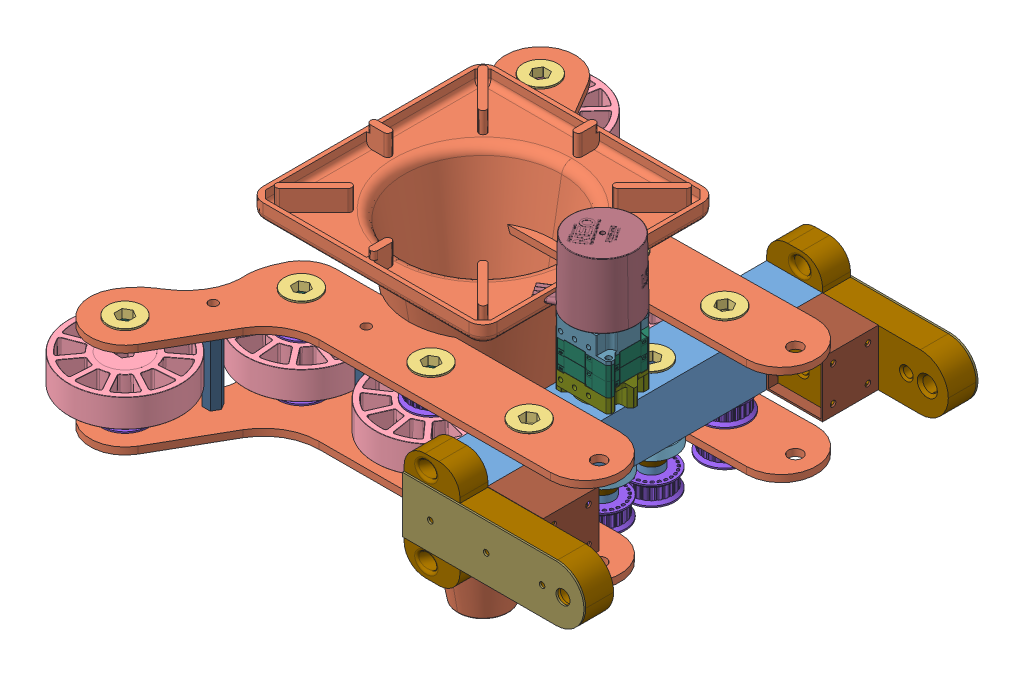
SolidWorks assembly Intake_Claw_2.0, configuration Default. Lengths in mm. (continued)
Mates (geometry in assembly coordinates): (continued)
- Concentric78: concentric anti-aligned: circle of am-2986 FR8ZZ Hex Bearing.step-11; circle of half_inch_hex_spacer_0.125inch-12
- Coincident81: coincident anti-aligned: plane of 24_tooth_5mmHTD_timing_belt_pulley_9mm-4 through (-63.197 63.4263 248.6341) normal (0 -1 0); circle of half_inch_hex_spacer_0.125inch-12
- Coincident83: coincident anti-aligned: plane of 24_tooth_5mmHTD_timing_belt_pulley_9mm-2 through (-230.4157 63.4263 364.5609) normal (0 -1 0); plane of half_inch_hex_spacer_0.125inch-9 through (-230.4157 63.4263 364.5609) normal (0 1 0)
- Coincident84: coincident anti-aligned: plane of 24_tooth_5mmHTD_timing_belt_pulley_9mm-14 through (-180.2715 63.4263 258.3256) normal (0 -1 0); plane of half_inch_hex_spacer_0.125inch-10 through (-180.2715 63.4263 258.3256) normal (0 1 0)
- Coincident85: coincident anti-aligned: plane of Intake_Plate_Assembly_2-2/am-2986 FR8ZZ Hex Bearing.step-11 through (-65.429 60.2513 76.6249) normal (0 1 0); plane of half_inch_hex_spacer_0.125inch-11 through (-63.3778 60.2513 58.8404) normal (0 -1 0)
- Concentric79: concentric anti-aligned: circle of Intake_Plate_Assembly_2-2/am-2986 FR8ZZ Hex Bearing.step-11; circle of half_inch_hex_spacer_0.125inch-11
- Coincident86: coincident anti-aligned: plane of 24_tooth_5mmHTD_timing_belt_pulley_9mm-12 through (-63.3778 63.4263 58.8404) normal (0 -1 0); plane of half_inch_hex_spacer_0.125inch-11 through (-63.3778 63.4263 58.8404) normal (0 1 0)
- Coincident87: coincident anti-aligned: plane of Intake_Plate_Assembly_2-2/am-2986 FR8ZZ Hex Bearing.step-18 through (-238.9399 60.2513 -29.6536) normal (0 1 0); plane of half_inch_hex_spacer_0.125inch-8 through (-234.0156 60.2513 -51.9922) normal (0 -1 0)
- Concentric80: concentric anti-aligned: circle of Intake_Plate_Assembly_2-2/am-2986 FR8ZZ Hex Bearing.step-18; circle of half_inch_hex_spacer_0.125inch-8
- Coincident88: coincident anti-aligned: plane of 24_tooth_5mmHTD_timing_belt_pulley_9mm-6 through (-234.0156 63.4263 -51.9922) normal (0 -1 0); plane of half_inch_hex_spacer_0.125inch-8 through (-234.0156 63.4263 -51.9922) normal (0 1 0)
- Coincident89: coincident anti-aligned: plane of Intake_Plate_Assembly_2-2/am-2986 FR8ZZ Hex Bearing.step-17 through (-182.8644 60.2513 73.5739) normal (0 1 0); plane of half_inch_hex_spacer_0.125inch-7 through (-180.6913 60.2513 52.683) normal (0 -1 0)
- Concentric81: concentric aligned: circle of Intake_Plate_Assembly_2-2/am-2986 FR8ZZ Hex Bearing.step-17; circle of half_inch_hex_spacer_0.125inch-7
- Coincident90: coincident anti-aligned: plane of 24_tooth_5mmHTD_timing_belt_pulley_9mm-5 through (-180.6913 63.4263 52.683) normal (0 -1 0); plane of half_inch_hex_spacer_0.125inch-7 through (-180.6913 63.4263 52.683) normal (0 1 0)
- Coincident95: coincident anti-aligned: plane of Claw_Crossbar-1 through (0 0 0) normal (0 0 -1); plane of Grabber_Spring_Mount-2 through (31.75 -4.7625 0) normal (0 0 1)
- Coincident97: coincident aligned: plane of Claw_Crossbar-1 through (50.8 0 304.8) normal (1 0 0); plane of Grabber_Spring_Mount-2 through (50.8 54.9275 -25.4) normal (1 0 0)
- Coincident101: coincident anti-aligned: plane of Intake_Plate_Assembly-1/am-2986 FR8ZZ Hex Bearing.step-5 through (23.441 -9.4513 78.9337) normal (0 -1 0); plane of half_inch_hex_spacer_0.125inch-19 through (25.4 -1.524 63.5) normal (0 1 0)
- Concentric82: concentric anti-aligned: circle of Intake_Plate_Assembly-1/am-2986 FR8ZZ Hex Bearing.step-5; circle of half_inch_hex_spacer_0.125inch-19
- Coincident102: coincident anti-aligned: plane of 24_tooth_5mmHTD_timing_belt_pulley_9mm-18 through (25.4 -4.699 63.5) normal (0 1 0); plane of half_inch_hex_spacer_0.125inch-19 through (25.4 -4.699 63.5) normal (0 -1 0)
- Concentric83: concentric aligned: cylinder of 24_tooth_5mmHTD_timing_belt_pulley_9mm-18 through (25.4 -22.479 63.5) axis (0 1 0) radius 21.082; circle of half_inch_hex_spacer_0.125inch-19
- Coincident103: coincident anti-aligned: plane of Intake_Plate_Assembly_2-1/am-2986 FR8ZZ Hex Bearing.step-16 through (24.1288 -9.4513 225.7945) normal (0 -1 0); plane of half_inch_hex_spacer_0.125inch-20 through (25.4 -1.524 241.3) normal (0 1 0)
- Concentric84: concentric aligned: circle of Intake_Plate_Assembly_2-1/am-2986 FR8ZZ Hex Bearing.step-16; circle of half_inch_hex_spacer_0.125inch-20
- Coincident104: coincident anti-aligned: plane of 24_tooth_5mmHTD_timing_belt_pulley_9mm-17 through (25.4 -4.699 241.3) normal (0 1 0); plane of half_inch_hex_spacer_0.125inch-20 through (25.4 -4.699 241.3) normal (0 -1 0)
- Concentric85: concentric anti-aligned: circle of 24_tooth_5mmHTD_timing_belt_pulley_9mm-17; circle of half_inch_hex_spacer_0.125inch-20
- Coincident105: coincident anti-aligned: plane of Intake_Plate_Assembly-1/am-2986 FR8ZZ Hex Bearing.step-11 through (-65.429 -9.4513 76.6249) normal (0 -1 0); plane of half_inch_hex_spacer_0.125inch-21 through (-63.4941 2.794 64.523) normal (0 1 0)
- Concentric86: concentric anti-aligned: circle of Intake_Plate_Assembly-1/am-2986 FR8ZZ Hex Bearing.step-11; circle of half_inch_hex_spacer_0.125inch-21
- Coincident106: coincident anti-aligned: plane of half_inch_hex_spacer_0.125inch-21 through (-63.4941 -0.381 64.523) normal (0 -1 0); plane of 24_tooth_5mmHTD_timing_belt_pulley_9mm-19 through (-63.4941 -0.381 64.523) normal (0 1 0)
- Concentric87: concentric anti-aligned: circle of half_inch_hex_spacer_0.125inch-21; circle of 24_tooth_5mmHTD_timing_belt_pulley_9mm-19
- Coincident107: coincident anti-aligned: plane of half_inch_hex_spacer_0.125inch-30 through (-63.4941 -18.161 64.523) normal (0 1 0); plane of 24_tooth_5mmHTD_timing_belt_pulley_9mm-19 through (-63.4941 -18.161 64.523) normal (0 -1 0)
- Concentric88: concentric anti-aligned: circle of half_inch_hex_spacer_0.125inch-30; circle of 24_tooth_5mmHTD_timing_belt_pulley_9mm-19
- Coincident108: coincident anti-aligned: plane of Intake_Plate_Assembly-1/am-2986 FR8ZZ Hex Bearing.step-12 through (-182.8644 -9.4513 73.5739) normal (0 -1 0); plane of half_inch_hex_spacer_0.125inch-22 through (-180.9613 2.794 65.8749) normal (0 1 0)
- Concentric89: concentric anti-aligned: circle of Intake_Plate_Assembly-1/am-2986 FR8ZZ Hex Bearing.step-12; circle of half_inch_hex_spacer_0.125inch-22
- Coincident109: coincident anti-aligned: plane of half_inch_hex_spacer_0.125inch-22 through (-180.9613 -0.381 65.8749) normal (0 -1 0); plane of 24_tooth_5mmHTD_timing_belt_pulley_9mm-20 through (-180.9613 -0.381 65.8749) normal (0 1 0)
- Concentric90: concentric anti-aligned: circle of half_inch_hex_spacer_0.125inch-22; circle of 24_tooth_5mmHTD_timing_belt_pulley_9mm-20
- Coincident110: coincident anti-aligned: plane of half_inch_hex_spacer_0.125inch-31 through (-180.9613 -18.161 65.8749) normal (0 1 0); plane of 24_tooth_5mmHTD_timing_belt_pulley_9mm-20 through (-180.9613 -18.161 65.8749) normal (0 -1 0)
- Concentric91: concentric anti-aligned: circle of half_inch_hex_spacer_0.125inch-31; circle of 24_tooth_5mmHTD_timing_belt_pulley_9mm-20
- Coincident111: coincident anti-aligned: plane of Intake_Plate_Assembly-1/am-2986 FR8ZZ Hex Bearing.step-3 through (-238.9399 -9.4513 -29.6536) normal (0 -1 0); plane of half_inch_hex_spacer_0.125inch-23 through (-240.8657 2.794 -35.1788) normal (0 1 0)
- Concentric92: concentric anti-aligned: circle of Intake_Plate_Assembly-1/am-2986 FR8ZZ Hex Bearing.step-3; circle of half_inch_hex_spacer_0.125inch-23
- Coincident112: coincident anti-aligned: plane of half_inch_hex_spacer_0.125inch-23 through (-240.8657 -0.381 -35.1788) normal (0 -1 0); plane of 24_tooth_5mmHTD_timing_belt_pulley_9mm-21 through (-240.8657 -0.381 -35.1788) normal (0 1 0)
- Concentric93: concentric anti-aligned: circle of half_inch_hex_spacer_0.125inch-23; circle of 24_tooth_5mmHTD_timing_belt_pulley_9mm-21
- Coincident113: coincident anti-aligned: circle of half_inch_hex_spacer_0.125inch-32; plane of 24_tooth_5mmHTD_timing_belt_pulley_9mm-21 through (-240.8657 -18.161 -35.1788) normal (0 -1 0)
- Concentric94: concentric anti-aligned: circle of half_inch_hex_spacer_0.125inch-32; circle of 24_tooth_5mmHTD_timing_belt_pulley_9mm-21
- Coincident114: coincident anti-aligned: plane of Intake_Plate_Assembly_2-1/am-2986 FR8ZZ Hex Bearing.step-18 through (-242.8184 -9.4513 322.6147) normal (0 -1 0); circle of half_inch_hex_spacer_0.125inch-24
- Concentric95: concentric anti-aligned: circle of Intake_Plate_Assembly_2-1/am-2986 FR8ZZ Hex Bearing.step-18; circle of half_inch_hex_spacer_0.125inch-24
- Coincident115: coincident anti-aligned: plane of half_inch_hex_spacer_0.125inch-24 through (-239.4221 -0.381 343.7898) normal (0 -1 0); plane of 24_tooth_5mmHTD_timing_belt_pulley_9mm-22 through (-239.4221 -0.381 343.7898) normal (0 1 0)
- Concentric96: concentric anti-aligned: circle of half_inch_hex_spacer_0.125inch-24; circle of 24_tooth_5mmHTD_timing_belt_pulley_9mm-22
- Coincident116: coincident anti-aligned: plane of half_inch_hex_spacer_0.125inch-29 through (-239.4221 -18.161 343.7898) normal (0 1 0); plane of 24_tooth_5mmHTD_timing_belt_pulley_9mm-22 through (-239.4221 -18.161 343.7898) normal (0 -1 0)
- Concentric97: concentric anti-aligned: circle of half_inch_hex_spacer_0.125inch-29; circle of 24_tooth_5mmHTD_timing_belt_pulley_9mm-22
- Coincident117: coincident anti-aligned: plane of Intake_Plate_Assembly_2-1/am-2986 FR8ZZ Hex Bearing.step-17 through (-182.211 -9.4513 221.9811) normal (0 -1 0); plane of half_inch_hex_spacer_0.125inch-25 through (-180.9742 2.794 241.8869) normal (0 1 0)
- Concentric98: concentric aligned: circle of Intake_Plate_Assembly_2-1/am-2986 FR8ZZ Hex Bearing.step-17; circle of half_inch_hex_spacer_0.125inch-25
- Coincident118: coincident anti-aligned: plane of half_inch_hex_spacer_0.125inch-25 through (-180.9742 -0.381 241.8869) normal (0 -1 0); plane of 24_tooth_5mmHTD_timing_belt_pulley_9mm-23 through (-180.9742 -0.381 241.8869) normal (0 1 0)
- Concentric99: concentric anti-aligned: circle of half_inch_hex_spacer_0.125inch-25; circle of 24_tooth_5mmHTD_timing_belt_pulley_9mm-23
- Coincident119: coincident anti-aligned: plane of half_inch_hex_spacer_0.125inch-28 through (-180.9742 -18.161 241.8869) normal (0 1 0); plane of 24_tooth_5mmHTD_timing_belt_pulley_9mm-23 through (-180.9742 -18.161 241.8869) normal (0 -1 0)
- Concentric100: concentric anti-aligned: circle of half_inch_hex_spacer_0.125inch-28; circle of 24_tooth_5mmHTD_timing_belt_pulley_9mm-23
- Coincident120: coincident anti-aligned: plane of Intake_Plate_Assembly_2-1/am-2986 FR8ZZ Hex Bearing.step-11 through (-64.7561 -9.4513 224.1518) normal (0 -1 0); plane of half_inch_hex_spacer_0.125inch-26 through (-63.4996 2.794 241.5528) normal (0 1 0)
- Concentric101: concentric anti-aligned: circle of Intake_Plate_Assembly_2-1/am-2986 FR8ZZ Hex Bearing.step-11; circle of half_inch_hex_spacer_0.125inch-26
- Coincident121: coincident anti-aligned: plane of half_inch_hex_spacer_0.125inch-26 through (-63.4996 -0.381 241.5528) normal (0 -1 0); plane of 24_tooth_5mmHTD_timing_belt_pulley_9mm-24 through (-63.4996 -0.381 241.5528) normal (0 1 0)
- Concentric102: concentric aligned: circle of Intake_Plate_Assembly_2-1/am-2986 FR8ZZ Hex Bearing.step-11; circle of 24_tooth_5mmHTD_timing_belt_pulley_9mm-24
- Coincident122: coincident anti-aligned: plane of half_inch_hex_spacer_0.125inch-27 through (-63.4996 -18.161 241.5528) normal (0 1 0); plane of 24_tooth_5mmHTD_timing_belt_pulley_9mm-24 through (-63.4996 -18.161 241.5528) normal (0 -1 0)
- Concentric103: concentric anti-aligned: circle of half_inch_hex_spacer_0.125inch-27; circle of 24_tooth_5mmHTD_timing_belt_pulley_9mm-24
- Coincident123: coincident anti-aligned: plane of 24_tooth_5mmHTD_timing_belt_pulley_9mm-18 through (25.4 -22.479 63.5) normal (0 -1 0); plane of half_inch_hex_spacer_0.125inch-33 through (25.4 -22.479 63.5) normal (0 1 0)
- Concentric104: concentric anti-aligned: circle of 24_tooth_5mmHTD_timing_belt_pulley_9mm-18; circle of half_inch_hex_spacer_0.125inch-33
- Coincident124: coincident anti-aligned: plane of 24_tooth_5mmHTD_timing_belt_pulley_9mm-17 through (25.4 -22.479 241.3) normal (0 -1 0); plane of half_inch_hex_spacer_0.125inch-34 through (25.4 -22.479 241.3) normal (0 1 0)
- Concentric105: concentric anti-aligned: circle of 24_tooth_5mmHTD_timing_belt_pulley_9mm-17; circle of half_inch_hex_spacer_0.125inch-34
- Coincident125: coincident anti-aligned: plane of half_inch_hex_spacer_0.125inch-27 through (-63.4996 -21.336 241.5528) normal (0 -1 0); plane of Intake_Plate_Assembly_2-4/am-2986 FR8ZZ Hex Bearing.step-11 through (-63.4848 -33.5813 239.6573) normal (0 1 0)
- Concentric106: concentric aligned: circle of 24_tooth_5mmHTD_timing_belt_pulley_9mm-17; circle of Intake_Plate_Assembly_2-4/am-2986 FR8ZZ Hex Bearing.step-16
- Coincident126: coincident aligned: plane of Intake_Plate_Assembly_2-1/Claw_Intake_Plates-3 through (75.6047 -1.5773 273.9833) normal (-0.018478 0 0.999829); plane of Intake_Plate_Assembly_2-4/Claw_Intake_Plates-3 through (75.6047 -33.6347 273.9833) normal (-0.018478 0 0.999829)
- Coincident127: coincident anti-aligned: plane of half_inch_hex_spacer_0.125inch-33 through (25.4 -25.654 63.5) normal (0 -1 0); plane of Intake_Plate_Assembly-3/am-2986 FR8ZZ Hex Bearing.step-5 through (25.4 -33.5813 63.5) normal (0 1 0)
- Concentric107: concentric anti-aligned: circle of half_inch_hex_spacer_0.125inch-33; circle of Intake_Plate_Assembly-3/am-2986 FR8ZZ Hex Bearing.step-5
- Coincident128: coincident aligned: plane of Intake_Plate_Assembly-1/Claw_Intake_Plates-3 through (77.0074 -7.9273 33.08) normal (0.025971 0 -0.999663); plane of Intake_Plate_Assembly-3/Claw_Intake_Plates-3 through (77.0074 -39.9847 33.08) normal (0.025971 0 -0.999663)
- Coincident130: coincident anti-aligned: plane of Intake_Plate_Assembly_2-1/Claw_Intake_Plates-3 through (-241.5471 -1.5773 338.1202) normal (0 1 0); plane of grabber_stand_off-1 through (-122.2369 -23.8023 241.7198) normal (0 -1 0)
- Concentric109: concentric anti-aligned: circle of Claw_Intake_Plates-3; circle of grabber_stand_off-1
- Coincident132: coincident anti-aligned: plane of Claw_Intake_Plates-3 through (-239.4221 52.3773 343.7898) normal (0 -1 0); plane of grabber_stand_off-3 through (-210.1981 52.3773 292.8384) normal (0 1 0)
- Concentric110: concentric anti-aligned: circle of Claw_Intake_Plates-3; circle of grabber_stand_off-3
- Coincident133: coincident anti-aligned: plane of Intake_Plate_Assembly_2-2/Claw_Intake_Plates-3 through (-236.9809 52.3773 -45.0872) normal (0 -1 0); plane of grabber_stand_off-5 through (-122.2277 50.6322 65.199) normal (0 1 0)
- Concentric111: concentric aligned: circle of Intake_Plate_Assembly_2-2/Claw_Intake_Plates-3; circle of grabber_stand_off-5
- Coincident134: coincident anti-aligned: plane of Intake_Plate_Assembly_2-2/Claw_Intake_Plates-3 through (-236.9809 52.3773 -45.0872) normal (0 -1 0); plane of grabber_stand_off-4 through (-210.9135 44.5398 15.3481) normal (0 1 0)
- Concentric112: concentric aligned: circle of Intake_Plate_Assembly_2-2/Claw_Intake_Plates-3; circle of grabber_stand_off-4
- Coincident136: coincident anti-aligned: plane of Claw_Crossbar-1 through (1.5875 1.5875 304.8) normal (0 1 0); plane of Grabber_Spring_Mount-2 through (48.5775 1.5875 0) normal (0 -1 0)
- Coincident137: coincident anti-aligned: plane of Claw_Crossbar-1 through (1.5875 1.5875 304.8) normal (0 1 0); plane of Grabber_Spring_Mount-1 through (49.2125 1.5875 304.8) normal (0 -1 0)
- Coincident138: coincident anti-aligned: plane of Claw_Crossbar-1 through (49.2125 1.5875 304.8) normal (-1 0 0); plane of Grabber_Spring_Mount-1 through (49.2125 48.5775 304.8) normal (1 0 0)
- Coincident139: coincident anti-aligned: plane of Claw_Crossbar-1 through (0 0 304.8) normal (0 0 1); plane of Grabber_Spring_Mount-1 through (32.385 54.9275 304.8) normal (0 0 -1)
- Coincident140: coincident aligned: plane of Claw_Crossbar-1 through (0 0 304.8) normal (0 -1 0); plane of Crossbar_Bracket-1 through (101.6 0 50.8) normal (0 -1 0)
- Coincident141: coincident anti-aligned: plane of Claw_Crossbar-1 through (50.8 0 304.8) normal (1 0 0); plane of Crossbar_Bracket-1 through (50.8 0 50.8) normal (-1 0 0)
- Coincident142: coincident: line of Claw_Crossbar-1 through (0 50.8 0) axis (0 0 1); plane of Crossbar_Bracket-1 through (101.6 0 0) normal (0 0 -1)
- Coincident143: coincident anti-aligned: plane of Claw_Crossbar-1 through (50.8 0 304.8) normal (1 0 0); plane of Crossbar_Bracket-2 through (50.8 0 304.8) normal (-1 0 0)
- Coincident144: coincident aligned: plane of Claw_Crossbar-1 through (0 0 304.8) normal (0 -1 0); plane of Crossbar_Bracket-2 through (101.6 0 304.8) normal (0 -1 0)
- Coincident145: coincident: line of Claw_Crossbar-1 through (0 0 304.8) axis (1 0 0); plane of Crossbar_Bracket-2 through (101.6 0 304.8) normal (0 0 1)
- Coincident146: coincident anti-aligned: plane of Grabber_Spring_Mount-1 through (32.385 54.9275 330.2) normal (0 0 1); plane of Claw_Pivot_Plate-1 through (140.335 25.0825 330.2) normal (0 0 -1)
- Concentric114: concentric anti-aligned: circle of Grabber_Spring_Mount-1; circle of Claw_Pivot_Plate-1
- Coincident147: coincident anti-aligned: plane of Grabber_Spring_Mount-2 through (31.75 -4.7625 -25.4) normal (0 0 -1); plane of Claw_Pivot_Plate-2 through (139.7 25.0825 -25.4) normal (0 0 1)
- Concentric115: concentric aligned: circle of Grabber_Spring_Mount-2; circle of Claw_Pivot_Plate-2
- Coincident148: coincident aligned: plane of Grabber_Spring_Mount-2 through (165.1 -0.3175 0) normal (0 -1 0); plane of Claw_Pivot_Plate-2 through (0 -0.3175 -25.4) normal (0 -1 0)
- Coincident149: coincident aligned: plane of Grabber_Spring_Mount-1 through (165.735 -0.3175 304.8) normal (0 -1 0); plane of Claw_Pivot_Plate-1 through (0.635 -0.3175 331.7875) normal (0 -1 0)
- Coincident151: coincident anti-aligned: plane of am-2986 FR8ZZ Hex Bearing.step-19 through (19.6679 -1.524 255.763) normal (0 -1 0); plane of half_inch_hex_spacer_0.125inch-20 through (25.4 -1.524 241.3) normal (0 1 0)
- Coincident152: coincident anti-aligned: plane of half_inch_hex_spacer_0.125inch-16 through (-63.4996 2.794 241.5528) normal (0 -1 0); plane of half_inch_hex_spacer_0.125inch-26 through (-63.4996 2.794 241.5528) normal (0 1 0)
- Coincident153: coincident anti-aligned: plane of half_inch_hex_spacer_0.125inch-17 through (-180.9742 2.794 241.8869) normal (0 -1 0); plane of half_inch_hex_spacer_0.125inch-25 through (-180.9742 2.794 241.8869) normal (0 1 0)
- Coincident154: coincident anti-aligned: plane of am-2986 FR8ZZ Hex Bearing.step-18 through (19.6679 -1.524 77.963) normal (0 -1 0); plane of half_inch_hex_spacer_0.125inch-19 through (25.4 -1.524 63.5) normal (0 1 0)
- Coincident155: coincident anti-aligned: plane of am-2986 FR8ZZ Hex Bearing.step-16 through (25.0352 52.324 47.9468) normal (0 1 0); plane of half_inch_hex_spacer_0.1875inch-1 through (25.4 52.324 63.5) normal (0 -1 0)
- Coincident157: coincident anti-aligned: plane of am-2986 FR8ZZ Hex Bearing.step-11 through (-63.4996 52.324 241.5528) normal (0 -1 0); plane of half_inch_hex_spacer_0.125inch-35 through (-63.4996 52.324 241.5528) normal (0 1 0)
- Concentric117: concentric anti-aligned: circle of am-3480 4IN 500Hex Bore Compliant Wheel REV2.STEP-3; circle of half_inch_hex_spacer_0.125inch-35
- Coincident158: coincident aligned: circle of 24_tooth_5mmHTD_timing_belt_pulley_9mm-15; plane of half_inch_hex_spacer_0.125inch-35 through (-63.4996 49.149 241.5528) normal (0 -1 0)
- Coincident159: coincident anti-aligned: plane of am-2986 FR8ZZ Hex Bearing.step-12 through (-180.9742 52.324 241.8869) normal (0 -1 0); plane of half_inch_hex_spacer_0.125inch-36 through (-180.9742 52.324 241.8869) normal (0 1 0)
- Concentric118: concentric anti-aligned: circle of 24_tooth_5mmHTD_timing_belt_pulley_9mm-3; circle of half_inch_hex_spacer_0.125inch-36
- Coincident160: coincident anti-aligned: plane of am-2986 FR8ZZ Hex Bearing.step-3 through (-239.4221 52.324 343.7898) normal (0 -1 0); plane of half_inch_hex_spacer_0.125inch-37 through (-239.4221 52.324 343.7898) normal (0 1 0)
- Concentric119: concentric aligned: circle of half_inch_hex_spacer_0.125inch-24; circle of half_inch_hex_spacer_0.125inch-37
- Coincident162: coincident anti-aligned: plane of half_inch_hex_spacer_0.125inch-18 through (-239.4221 2.794 343.7898) normal (0 -1 0); plane of half_inch_hex_spacer_0.125inch-24 through (-239.4221 2.794 343.7898) normal (0 1 0)
- Coincident163: coincident aligned: circle of 24_tooth_5mmHTD_timing_belt_pulley_9mm-13; plane of half_inch_hex_spacer_0.125inch-39 through (-180.9613 49.149 65.8749) normal (0 -1 0)
- Concentric120: concentric anti-aligned: circle of 24_tooth_5mmHTD_timing_belt_pulley_9mm-13; circle of half_inch_hex_spacer_0.125inch-39
- Coincident164: coincident aligned: circle of 24_tooth_5mmHTD_timing_belt_pulley_9mm-16; plane of half_inch_hex_spacer_0.125inch-38 through (-63.4941 49.149 64.523) normal (0 -1 0)
- Concentric121: concentric anti-aligned: circle of 24_tooth_5mmHTD_timing_belt_pulley_9mm-16; circle of half_inch_hex_spacer_0.125inch-38
- Coincident165: coincident anti-aligned: plane of half_inch_hex_spacer_0.125inch-13 through (-63.4941 2.794 64.523) normal (0 -1 0); plane of half_inch_hex_spacer_0.125inch-21 through (-63.4941 2.794 64.523) normal (0 1 0)
- Coincident166: coincident anti-aligned: plane of half_inch_hex_spacer_0.125inch-15 through (-240.8657 2.794 -35.1788) normal (0 -1 0); plane of half_inch_hex_spacer_0.125inch-23 through (-240.8657 2.794 -35.1788) normal (0 1 0)
- Coincident167: coincident anti-aligned: plane of half_inch_hex_spacer_0.125inch-14 through (-180.9613 2.794 65.8749) normal (0 -1 0); plane of half_inch_hex_spacer_0.125inch-22 through (-180.9613 2.794 65.8749) normal (0 1 0)
- Concentric122: concentric aligned: circle of Claw_Intake_Plates-4; circle of am-2986 FR8ZZ Hex Bearing.step-20
- Coincident168: coincident anti-aligned: plane of Claw_Intake_Plates-4 through (-239.4221 -27.7393 343.7898) normal (0 -1 0); plane of am-2986 FR8ZZ Hex Bearing.step-20 through (39.37 -27.7393 241.3) normal (0 1 0)
- Coincident169: coincident anti-aligned: plane of Claw_Intake_Plates-4 through (-239.4221 -27.7393 343.7898) normal (0 -1 0); plane of am-2986 FR8ZZ Hex Bearing.step-21 through (-52.0402 -27.7393 233.5627) normal (0 1 0)
- Coincident170: coincident anti-aligned: plane of Claw_Intake_Plates-4 through (-239.4221 -27.7393 343.7898) normal (0 -1 0); plane of am-2986 FR8ZZ Hex Bearing.step-22 through (-167.0042 -27.7393 241.8869) normal (0 1 0)
- Concentric123: concentric aligned: circle of Claw_Intake_Plates-4; circle of am-2986 FR8ZZ Hex Bearing.step-22
- Coincident171: coincident anti-aligned: plane of Claw_Intake_Plates-4 through (-239.4221 -27.7393 343.7898) normal (0 -1 0); plane of am-2986 FR8ZZ Hex Bearing.step-23 through (-225.4521 -27.7393 343.7898) normal (0 1 0)
- Concentric124: concentric anti-aligned: circle of Claw_Intake_Plates-4; cone of am-2986 FR8ZZ Hex Bearing.step-23 through (-239.4221 -29.1363 343.7898) axis (0 -1 0)
- Coincident173: coincident aligned: plane of Claw_Intake_Plates-3 through (76.2901 58.7273 272.9054) normal (0.002844 0 0.999996); plane of Claw_Intake_Plates-4 through (76.2901 -21.3893 272.9054) normal (0.002844 0 0.999996)
- Coincident174: coincident anti-aligned: plane of half_inch_hex_spacer_0.125inch-29 through (-239.4221 -21.336 343.7898) normal (0 -1 0); plane of am-2986 FR8ZZ Hex Bearing.step-23 through (-239.4221 -21.336 343.7898) normal (0 1 0)
- Concentric125: concentric anti-aligned: circle of half_inch_hex_spacer_0.125inch-20; circle of am-2986 FR8ZZ Hex Bearing.step-20
- Concentric126: concentric aligned: circle of am-2986 FR8ZZ Hex Bearing.step-19; circle of 24_tooth_5mmHTD_timing_belt_pulley_9mm-17
- Coincident175: coincident anti-aligned: plane of Claw_Intake_Plates-6 through (-240.8657 -32.0573 -35.1788) normal (0 -1 0); plane of am-2986 FR8ZZ Hex Bearing.step-24 through (39.37 -32.0573 63.5) normal (0 1 0)
- Concentric127: concentric anti-aligned: circle of Claw_Intake_Plates-6; circle of am-2986 FR8ZZ Hex Bearing.step-24
- Coincident176: coincident anti-aligned: circle of Claw_Intake_Plates-6; plane of am-2986 FR8ZZ Hex Bearing.step-25 through (-49.5241 -32.0573 64.523) normal (0 1 0)
- Concentric128: concentric aligned: circle of Claw_Intake_Plates-6; circle of am-2986 FR8ZZ Hex Bearing.step-25
- Coincident177: coincident anti-aligned: plane of Claw_Intake_Plates-6 through (-240.8657 -32.0573 -35.1788) normal (0 -1 0); plane of am-2986 FR8ZZ Hex Bearing.step-27 through (-166.9913 -32.0573 65.8749) normal (0 1 0)
- Concentric129: concentric aligned: circle of Claw_Intake_Plates-6; circle of am-2986 FR8ZZ Hex Bearing.step-27
- Coincident178: coincident anti-aligned: plane of Claw_Intake_Plates-6 through (-240.8657 -32.0573 -35.1788) normal (0 -1 0); plane of am-2986 FR8ZZ Hex Bearing.step-26 through (-226.8957 -32.0573 -35.1788) normal (0 1 0)
- Concentric130: concentric anti-aligned: circle of Claw_Intake_Plates-6; circle of am-2986 FR8ZZ Hex Bearing.step-26
- Coincident179: coincident anti-aligned: plane of Claw_Intake_Plates-5 through (-240.8657 58.7273 -35.1788) normal (0 1 0); plane of am-2986 FR8ZZ Hex Bearing.step-28 through (39.37 58.7273 63.5) normal (0 -1 0)
- Concentric131: concentric anti-aligned: circle of Claw_Intake_Plates-5; circle of am-2986 FR8ZZ Hex Bearing.step-28
- Coincident180: coincident anti-aligned: plane of Claw_Intake_Plates-5 through (-240.8657 58.7273 -35.1788) normal (0 1 0); plane of am-2986 FR8ZZ Hex Bearing.step-29 through (-49.5241 58.7273 64.523) normal (0 -1 0)
- Concentric132: concentric aligned: circle of Claw_Intake_Plates-5; circle of am-2986 FR8ZZ Hex Bearing.step-29
- Coincident181: coincident anti-aligned: plane of Claw_Intake_Plates-5 through (-240.8657 58.7273 -35.1788) normal (0 1 0); plane of am-2986 FR8ZZ Hex Bearing.step-30 through (-166.9913 58.7273 65.8749) normal (0 -1 0)
- Concentric133: concentric aligned: circle of Claw_Intake_Plates-5; circle of am-2986 FR8ZZ Hex Bearing.step-30
- Coincident182: coincident anti-aligned: plane of Claw_Intake_Plates-5 through (-240.8657 58.7273 -35.1788) normal (0 1 0); plane of am-2986 FR8ZZ Hex Bearing.step-31 through (-226.8957 58.7273 -35.1788) normal (0 -1 0)
- Concentric134: concentric anti-aligned: circle of Claw_Intake_Plates-5; circle of am-2986 FR8ZZ Hex Bearing.step-31
- Coincident183: coincident anti-aligned: plane of half_inch_hex_spacer_0.125inch-39 through (-180.9613 52.324 65.8749) normal (0 1 0); plane of am-2986 FR8ZZ Hex Bearing.step-30 through (-180.9613 52.324 65.8749) normal (0 -1 0)
- Concentric135: concentric aligned: circle of half_inch_hex_spacer_0.1875inch-1; circle of am-2986 FR8ZZ Hex Bearing.step-28
- Concentric136: concentric anti-aligned: circle of am-2986 FR8ZZ Hex Bearing.step-16; circle of am-2986 FR8ZZ Hex Bearing.step-28
- Coincident184: coincident anti-aligned: plane of half_inch_hex_spacer_0.125inch-33 through (25.4 -25.654 63.5) normal (0 -1 0); plane of am-2986 FR8ZZ Hex Bearing.step-24 through (25.4 -25.654 63.5) normal (0 1 0)
- Concentric137: concentric aligned: circle of half_inch_hex_spacer_0.125inch-33; circle of am-2986 FR8ZZ Hex Bearing.step-24
- Concentric138: concentric aligned: circle of am-2986 FR8ZZ Hex Bearing.step-18; circle of half_inch_hex_spacer_0.125inch-19
- Coincident185: coincident aligned: plane of Claw_Intake_Plates-5 through (75.8313 52.3773 31.1675) normal (-0.011508 0 -0.999934); plane of Claw_Intake_Plates-6 through (75.8313 -32.0573 31.1675) normal (-0.011508 0 -0.999934)
- Concentric139: concentric anti-aligned: circle of am-3480 4IN 500Hex Bore Compliant Wheel REV2.STEP-3; circle of am-2986 FR8ZZ Hex Bearing.step-21
- Concentric142: concentric anti-aligned: circle of Claw_Intake_Plates-4; circle of am-2986 FR8ZZ Hex Bearing.step-21
- Concentric143: concentric aligned: circle of half_inch_hex_spacer_0.125inch-16; circle of half_inch_hex_spacer_0.125inch-27
- Concentric144: concentric aligned: circle of half_inch_hex_spacer_0.125inch-16; circle of half_inch_hex_spacer_0.125inch-26
- Concentric145: concentric aligned: circle of half_inch_hex_spacer_0.125inch-28; circle of am-2986 FR8ZZ Hex Bearing.step-22
- Coincident190: coincident aligned: circle of half_inch_hex_spacer_0.125inch-17; circle of half_inch_hex_spacer_0.125inch-25
- Concentric146: concentric aligned: circle of half_inch_hex_spacer_0.125inch-29; circle of am-2986 FR8ZZ Hex Bearing.step-23
- Coincident191: coincident aligned: circle of half_inch_hex_spacer_0.125inch-18; circle of half_inch_hex_spacer_0.125inch-24
- Concentric147: concentric anti-aligned: circle of half_inch_hex_spacer_0.125inch-30; circle of am-2986 FR8ZZ Hex Bearing.step-25
- Concentric148: concentric aligned: circle of half_inch_hex_spacer_0.125inch-13; circle of am-2986 FR8ZZ Hex Bearing.step-25
- Concentric149: concentric aligned: circle of am-3480 4IN 500Hex Bore Compliant Wheel REV2.STEP-4; circle of am-2986 FR8ZZ Hex Bearing.step-25
- Concentric150: concentric anti-aligned: circle of half_inch_hex_spacer_0.125inch-38; circle of am-2986 FR8ZZ Hex Bearing.step-29
- Concentric151: concentric anti-aligned: circle of half_inch_hex_spacer_0.125inch-39; circle of am-2986 FR8ZZ Hex Bearing.step-30
- Concentric152: concentric anti-aligned: circle of half_inch_hex_spacer_0.125inch-31; circle of am-2986 FR8ZZ Hex Bearing.step-27
- Concentric153: concentric anti-aligned: circle of half_inch_hex_spacer_0.125inch-14; circle of am-2986 FR8ZZ Hex Bearing.step-27
- Concentric154: concentric aligned: circle of grabber_stand_off-5; circle of Claw_Intake_Plates-6
- Concentric155: concentric aligned: circle of grabber_stand_off-4; circle of Claw_Intake_Plates-6
- Concentric156: concentric anti-aligned: circle of half_inch_hex_spacer_0.125inch-32; circle of am-2986 FR8ZZ Hex Bearing.step-26
- Concentric157: concentric anti-aligned: circle of half_inch_hex_spacer_0.125inch-15; circle of am-2986 FR8ZZ Hex Bearing.step-26
- Coincident192: coincident anti-aligned: plane of am-2986 FR8ZZ Hex Bearing.step-13 through (19.6679 -1.524 144.638) normal (0 -1 0); plane of half_inch_hex_spacer_0.125inch-1 through (25.4 -1.524 130.175) normal (0 1 0)
- Coincident193: coincident anti-aligned: plane of Claw_Drive_Gear-1 through (25.4 -4.699 130.175) normal (0 1 0); plane of half_inch_hex_spacer_0.125inch-1 through (25.4 -4.699 130.175) normal (0 -1 0)
- Concentric158: concentric aligned: circle of Claw_Crossbar-1; circle of am-2986 FR8ZZ Hex Bearing.step-32
- Coincident195: coincident anti-aligned: plane of Claw_Crossbar-1 through (0 0 304.8) normal (0 -1 0); plane of am-2986 FR8ZZ Hex Bearing.step-32 through (18.4113 0 186.7212) normal (0 1 0)
- Coincident196: coincident anti-aligned: plane of half_inch_hex_spacer_0.125inch-2 through (25.4 -1.524 174.625) normal (0 1 0); plane of am-2986 FR8ZZ Hex Bearing.step-32 through (17.6171 -1.524 188.0958) normal (0 -1 0)
- Coincident197: coincident anti-aligned: plane of Claw_Drive_Gear-2 through (25.4 -4.699 174.625) normal (0 1 0); plane of half_inch_hex_spacer_0.125inch-2 through (25.4 -4.699 174.625) normal (0 -1 0)
- Concentric159: concentric aligned: circle of Claw_Crossbar-1; circle of Neo_with_2_Stage_Gearbox-1/REV-21-2104.step-1
- Coincident200: coincident anti-aligned: plane of Claw_Crossbar-1 through (0 50.8 304.8) normal (0 1 0); plane of Neo_with_2_Stage_Gearbox-1/REV-21-2104.step-1 through (25.4 50.8 174.625) normal (0 -1 0)
- Parallel9: parallel aligned: plane of Claw_Crossbar-1 through (0 0 304.8) normal (-1 0 0); plane of Neo_with_2_Stage_Gearbox-1/REV-21-2103.step-1 through (0 82.55 149.225) normal (-1 0 0)
- Coincident202: coincident anti-aligned: circle of Claw_Drive_Gear-2; plane of half_inch_hex_spacer_0.125inch-2 through (25.4 -4.699 174.625) normal (0 -1 0)
- Concentric160: concentric aligned: circle of Claw_Drive_Gear-2; circle of half_inch_hex_spacer_0.125inch-2
- Concentric161: concentric anti-aligned: circle of half_inch_hex_spacer_0.125inch-2; circle of am-2986 FR8ZZ Hex Bearing.step-32
- Coincident203: coincident anti-aligned: plane of am-2986 FR8ZZ Hex Bearing.step-20 through (40.9575 -29.2633 241.3) normal (0 -1 0); plane of half_inch_hex_spacer_0.125inch-41 through (25.4 -29.2633 241.3) normal (0 1 0)
- Concentric162: concentric anti-aligned: circle of am-2986 FR8ZZ Hex Bearing.step-20; circle of half_inch_hex_spacer_0.125inch-41
- Coincident204: coincident anti-aligned: plane of am-2986 FR8ZZ Hex Bearing.step-24 through (40.9575 -33.5813 63.5) normal (0 -1 0); plane of half_inch_hex_spacer_0.125inch-40 through (25.4 -33.5813 63.5) normal (0 1 0)
- Concentric163: concentric anti-aligned: circle of am-2986 FR8ZZ Hex Bearing.step-24; circle of half_inch_hex_spacer_0.125inch-40
- Coincident205: coincident aligned: plane of half_inch_hex_spacer_0.125inch-40 through (25.4 -36.7563 63.5) normal (0 -1 0); circle of 24_tooth_5mmHTD_timing_belt_pulley_9mm-25
- Concentric164: concentric anti-aligned: circle of half_inch_hex_spacer_0.125inch-40; circle of 24_tooth_5mmHTD_timing_belt_pulley_9mm-25
- Coincident206: coincident aligned: plane of half_inch_hex_spacer_0.125inch-41 through (25.4 -32.4383 241.3) normal (0 -1 0); circle of 24_tooth_5mmHTD_timing_belt_pulley_9mm-26
- Concentric165: concentric anti-aligned: circle of half_inch_hex_spacer_0.125inch-41; circle of 24_tooth_5mmHTD_timing_belt_pulley_9mm-26
- Coincident207: coincident anti-aligned: plane of Claw_Drive_Gear-1 through (25.4 -14.1478 130.175) normal (0 -1 0); plane of half_inch_hex_spacer_0.5inch-1 through (25.4 -14.1478 130.175) normal (0 1 0)
- Concentric166: concentric aligned: circle of Claw_Drive_Gear-1; circle of half_inch_hex_spacer_0.5inch-1
- Coincident208: coincident anti-aligned: plane of half_inch_hex_spacer_0.5inch-1 through (25.4 -26.8478 130.175) normal (0 -1 0); plane of half_inch_hex_spacer_0.25inch-1 through (25.4 -26.8478 130.175) normal (0 1 0)
- Concentric167: concentric aligned: circle of half_inch_hex_spacer_0.5inch-1; circle of half_inch_hex_spacer_0.25inch-1
- Coincident210: coincident aligned: circle of 24_tooth_5mmHTD_timing_belt_pulley_9mm-9; plane of half_inch_hex_spacer_0.25inch-1 through (25.4 -33.1978 130.175) normal (0 -1 0)
- Concentric168: concentric anti-aligned: circle of 24_tooth_5mmHTD_timing_belt_pulley_9mm-9; circle of half_inch_hex_spacer_0.25inch-1
- Coincident211: coincident anti-aligned: plane of Claw_Drive_Gear-2 through (25.4 -14.1478 174.625) normal (0 -1 0); plane of half_inch_hex_spacer_0.5inch-2 through (25.4 -14.1478 174.625) normal (0 1 0)
- Concentric169: concentric aligned: circle of Claw_Drive_Gear-2; circle of half_inch_hex_spacer_0.5inch-2
- Coincident212: coincident anti-aligned: plane of half_inch_hex_spacer_0.5inch-2 through (25.4 -26.8478 174.625) normal (0 -1 0); plane of half_inch_hex_spacer_0.25inch-2 through (25.4 -26.8478 174.625) normal (0 1 0)
- Coincident213: coincident aligned: circle of half_inch_hex_spacer_0.5inch-2; circle of half_inch_hex_spacer_0.25inch-2
- Coincident214: coincident aligned: circle of 24_tooth_5mmHTD_timing_belt_pulley_9mm-8; plane of half_inch_hex_spacer_0.25inch-2 through (25.4 -33.1978 174.625) normal (0 -1 0)
- Concentric170: concentric anti-aligned: circle of 24_tooth_5mmHTD_timing_belt_pulley_9mm-8; circle of half_inch_hex_spacer_0.25inch-2
- Parallel10: parallel aligned: plane of Claw_Intake_Plates-4 through (-239.4221 -27.7393 343.7898) normal (0 -1 0); plane of am-4700_syc Cone-1 through (-200.025 109.5273 57.8461) normal (0 -1 0)
- Coincident217: coincident anti-aligned: plane of Claw_Crossbar-1 through (0 0 304.8) normal (-1 0 0); plane of am-4700_syc Cone-1 through (0 109.5273 57.8461) normal (1 0 0)
- Distance1: distance = 50.8 mm anti-aligned: plane of am-4700_syc Cone-1 through (-200.025 109.5273 57.8461) normal (0 -1 0); plane of Claw_Intake_Plates-3 through (-239.4221 58.7273 343.7898) normal (0 1 0)
- Distance2: distance = 73.9164 mm aligned: plane of am-4700_syc Cone-1 through (-200.025 109.5273 257.8711) normal (0 0 1); plane of Claw_Pivot_Plate-1 through (140.335 25.0825 331.7875) normal (0 0 1)
